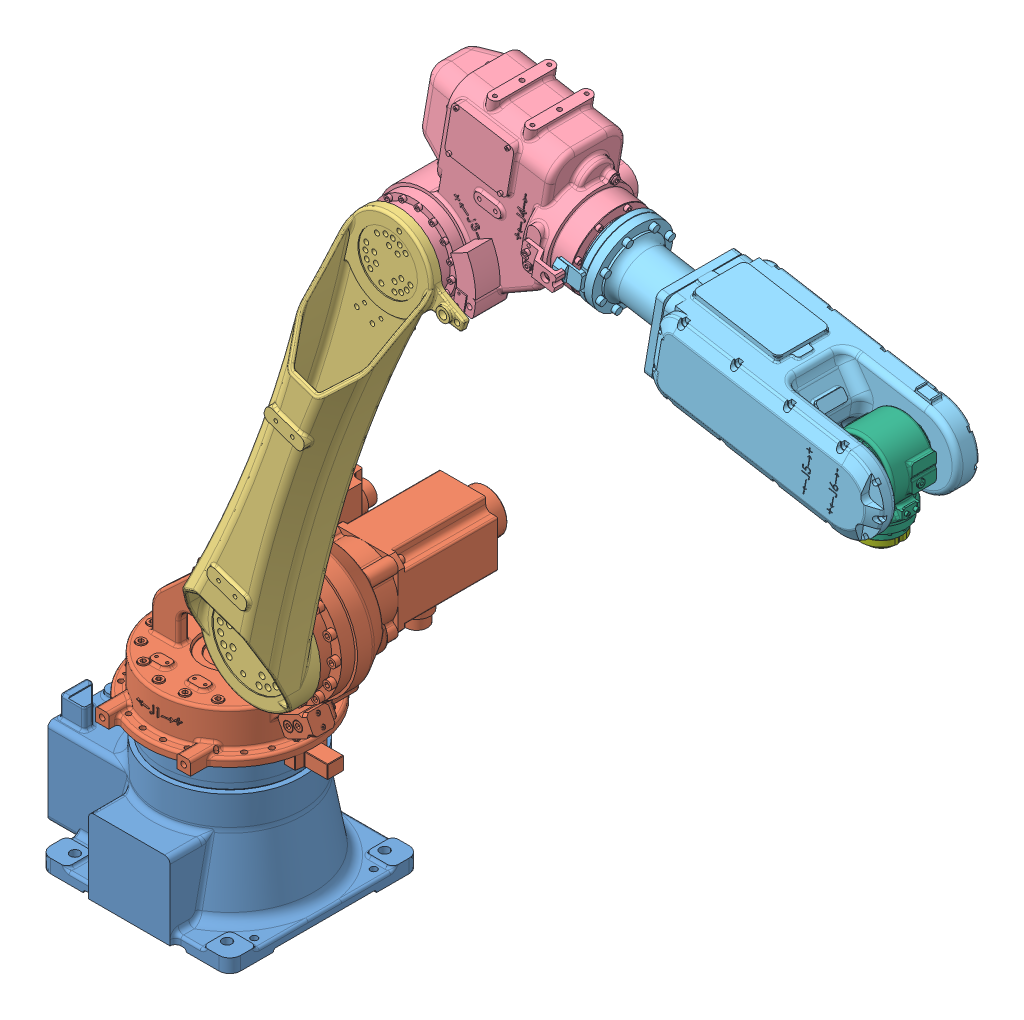
SolidWorks assembly ER20-C10, configuration 默认. Lengths in mm.
Overall size (1530.48 1536.94 537.9).
7 component instances, 7 part files, 21 mates.
Components (placement in the parent):
- ER20底座-1: ER20底座 [默认] at origin size (413 328.35 365)
- ER20转座-1: ER20转座 [默认] at (0 91.5931 0) size (440 420.81 463)
- ER20大臂-1: ER20大臂 [默认] at (170 504 319.9) x (-0.945729 0.324955 0) z (0 0 -1) size (235.15 960 175)
- ER20小臂-1: ER20小臂 [默认] at (423.4652 1241.6689 -44.55) x (0.985593 -0.169132 0) z (0 0 1) size (348.5 370 298)
- ER20小臂杆-1: ER20小臂杆 [默认] at (19.6118 1453.0181 0) x (0.985593 -0.169132 0) z (0 0 1) size (611.64 164.3 202.56)
- ER20手腕-1: ER20手腕 [默认] at (1199.1514 1250.6045 0) x (0 -1 0) z (0 0 -1) size (176.5 129 123.7)
- ER20末端法兰-1: ER20末端法兰 [默认] at (1199.1514 1250.6045 0) x (0 -1 0) z (0 0 -1) size (22 73.5 75)
Mates (geometry in assembly coordinates):
- 重合1: coincident: plane of ER20底座-1 through (0 0 0) normal (0 0 1); plane of assembly through (0 0 0) normal (0 0 1)
- 重合2: coincident: plane of ER20底座-1 through (0 0 0) normal (0 1 0); plane of assembly through (0 0 0) normal (0 1 0)
- 重合3: coincident aligned: plane of ER20底座-1 through (0 0 0) normal (1 0 0); plane of assembly through (0 0 0) normal (1 0 0)
- 距离1: distance = 349 mm anti-aligned: plane of ER20转座-1 through (-50 349 0) normal (0 1 0); plane of ER20底座-1 through (-175 0 175) normal (0 -1 0)
- 同心1: concentric aligned: cylinder of ER20转座-1 through (0 269 0) axis (0 -1 0) radius 135; cylinder of ER20底座-1 through (0 206.4 0) axis (0 -1 0) radius 125.25
- 重合5: coincident aligned: plane of ER20底座-1 through (0 0 0) normal (0 0 1); plane of ER20转座-1 through (0 91.5931 0) normal (0 0 1)
- 距离2: distance = 3.9 mm anti-aligned: plane of ER20大臂-1 through (170 504 102.9) normal (0 0 -1); plane of ER20转座-1 through (250 504 99) normal (0 0 1)
- 同心2: concentric anti-aligned: cylinder of ER20转座-1 through (170 504 27.9) axis (0 0 -1) radius 93; cylinder of ER20大臂-1 through (170 504 119.9) axis (0 0 1) radius 100
- 角度1: planar angle = 1.570796 rad aligned: plane of ER20大臂-1 through (170 504 319.9) normal (-1 0 0); plane of ER20转座-1 through (0 91.5931 0) normal (0 1 0)
- 距离3: distance = 5.7 mm anti-aligned: plane of ER20大臂-1 through (423.4652 1241.6689 113.4) normal (0 0 -1); plane of ER20小臂-1 through (481.6152 1231.6901 107.7) normal (0 0 1)
- 同心3: concentric aligned: cylinder of ER20大臂-1 through (423.4652 1241.6689 119.9) axis (0 0 1) radius 80; cylinder of ER20小臂-1 through (423.4652 1241.6689 113.4) axis (0 0 1) radius 68
- 距离4: distance = 14 mm anti-aligned: plane of ER20小臂-1 through (692.878 1289.1554 -27.5) normal (0.985593 -0.169132 0); plane of ER20小臂杆-1 through (714.7322 1333.7327 0) normal (-0.985593 0.169132 0)
- 同心4: concentric aligned: cylinder of ER20小臂-1 through (704.8763 1335.424 0) axis (0.985593 -0.169132 0) radius 73.5; cylinder of ER20小臂杆-1 through (714.7322 1333.7327 0) axis (0.985593 -0.169132 0) radius 73.5
- 平行2: parallel aligned: plane of ER20小臂-1 through (423.4652 1241.6689 -44.55) normal (0 0 1); plane of ER20小臂杆-1 through (19.6118 1453.0181 0) normal (0 0 1)
- 平行3: parallel aligned: plane of ER20大臂-1; plane of ER20小臂-1 through (170 1284 -44.55) normal (0 1 0)
- 重合12: coincident anti-aligned: plane of ER20小臂杆-1 through (19.6118 1453.0181 0) normal (0 0 1); plane of ER20手腕-1 through (1199.1514 1250.6045 0) normal (0 0 -1)
- 同心5: concentric aligned: cylinder of ER20小臂杆-1 through (1199.1514 1250.6045 52) axis (0 0 -1) radius 52; cylinder of ER20手腕-1 through (1199.1514 1250.6045 37.0073) axis (0 0 -1) radius 52
- 同心7: concentric aligned: cylinder of ER20手腕-1 through (1199.1514 1187.1045 0) axis (0 1 0) radius 37.5; cylinder of ER20末端法兰-1 through (1199.1514 1147.6045 0) axis (0 1 0) radius 37.5
- 重合14: coincident anti-aligned: plane of ER20手腕-1 through (1199.1514 1147.6045 -37.5) normal (0 -1 0); plane of ER20末端法兰-1 through (1171.4514 1147.6045 0) normal (0 1 0)
- 重合15: coincident aligned: plane of ER20手腕-1 through (1199.1514 1250.6045 0) normal (0 0 -1); plane of ER20末端法兰-1 through (1199.1514 1250.6045 0) normal (0 0 -1)
- 平行4: parallel: line of ER20底座-1 through (0 267 0) axis (0 -1 0); plane of ER20手腕-1
